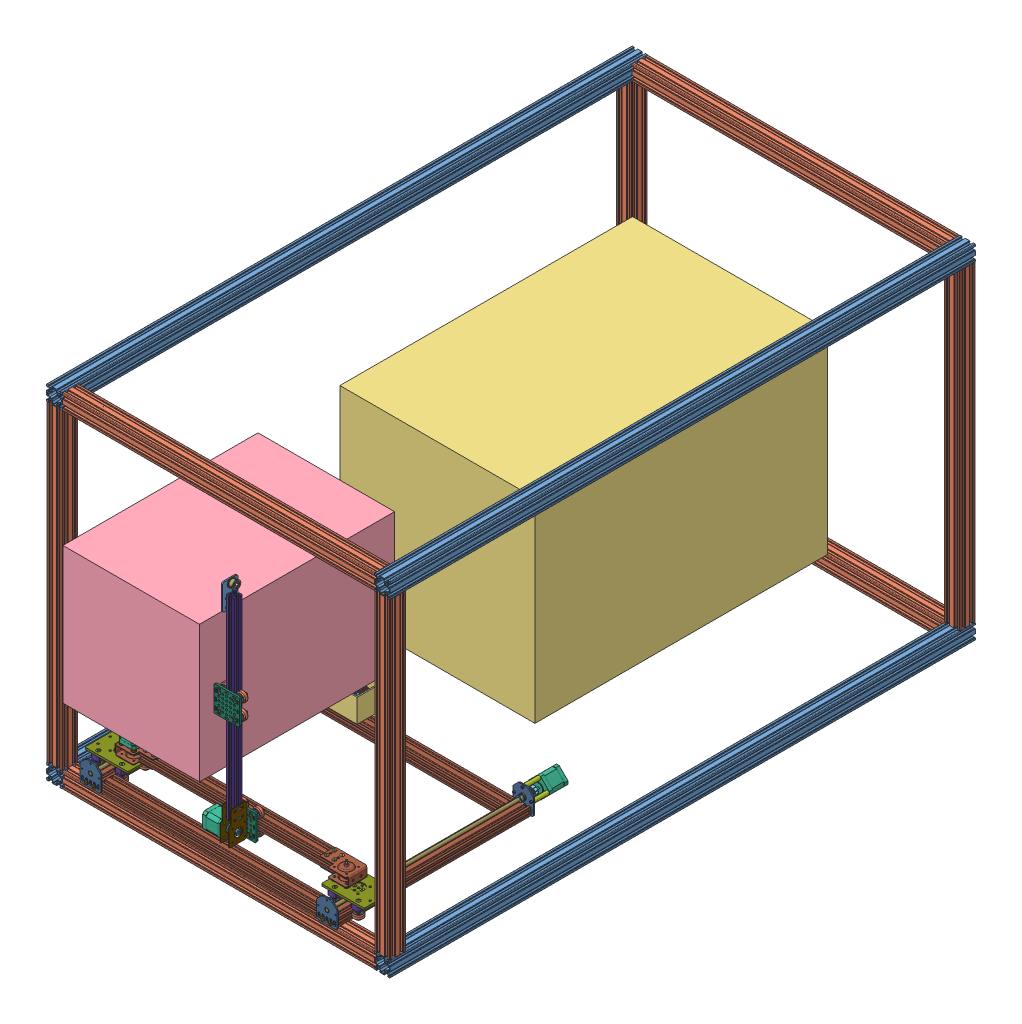
SolidWorks assembly box, configuration 預設. Lengths in mm.
Overall size (880 880 1515.78).
295 component instances, 42 part files, 42 mates.
Components (placement in the parent):
- V-Slot 40x40x1500 Linear Rail-1: V-Slot 40x40x1500 Linear Rail [Default] at (-19.0751 -0.7358 750) size (40 40 1500)
- V-Slot 40x40x1500 Linear Rail-2: V-Slot 40x40x1500 Linear Rail [Default] at (-19.0751 -840.7358 750) size (40 40 1500)
- V-Slot 40x40x1000 Linear Rail-1: V-Slot 40x40x1000 Linear Rail [40 x 40 x 800] at (-19.0751 -820.7358 2230) x (0 0 1) z (0 1 0) size (40 40 800)
- V-Slot 40x40x1000 Linear Rail-2: V-Slot 40x40x1000 Linear Rail [40 x 40 x 800] at (-19.0751 -820.7358 770) x (1 0 0) z (0 1 0) size (40 40 800)
- V-Slot 40x40x1000 Linear Rail-3: V-Slot 40x40x1000 Linear Rail [40 x 40 x 800] at (800.9249 -840.7358 2230) x (0 0 1) z (-1 0 0) size (40 40 800)
- V-Slot 40x40x1000 Linear Rail-4: V-Slot 40x40x1000 Linear Rail [40 x 40 x 800] at (800.9249 -0.7358 2230) x (0 0 1) z (-1 0 0) size (40 40 800)
- V-Slot 40x40x1000 Linear Rail-7: V-Slot 40x40x1000 Linear Rail [40 x 40 x 800] at (820.9249 -20.7358 2230) x (1 0 0) z (0 -1 0) size (40 40 800)
- V-Slot 40x40x1000 Linear Rail-8: V-Slot 40x40x1000 Linear Rail [40 x 40 x 800] at (800.9249 -840.7358 770) x (0 0 1) z (-1 0 0) size (40 40 800)
- V-Slot 40x40x1000 Linear Rail-9: V-Slot 40x40x1000 Linear Rail [40 x 40 x 800] at (820.9249 -820.7358 770) x (1 0 0) z (0 1 0) size (40 40 800)
- V-Slot 40x40x1000 Linear Rail-10: V-Slot 40x40x1000 Linear Rail [40 x 40 x 800] at (800.9249 -0.7358 770) x (0 0 1) z (-1 0 0) size (40 40 800)
- V-Slot 40x40x1500 Linear Rail-5: V-Slot 40x40x1500 Linear Rail [Default] at (820.9249 -840.7358 750) size (40 40 1500)
- V-Slot 40x40x1500 Linear Rail-6: V-Slot 40x40x1500 Linear Rail [Default] at (820.9249 -0.7358 750) size (40 40 1500)
- frige-2: frige [RS-5075G] at (307.8977 -579.3938 788.5) size (500 500 750)
- oven-1: oven [預設] at (0.9249 -15184.575 11029.75) x (0 -1 0) z (1 0 0) size (350 500 350)
- keg-1: keg [12L] at (296.649 -568.3878 823.5037) size (226.6 226.6 413)
- manipulator2-1: manipulator2 [預設] at (654.9752 -796.101 2551.2052) x (-0.998451 -0.052967 0.017023) z (-0.017075 0.000534 -0.999854) size (716.52 632.64 604.45) (flexible)
  - Button Head Socket Cap Screw M3-1: Button Head Socket Cap Screw M3 [M3 x 17] at (-17.8347 8.2677 364.2512) x (0.052967 -0.998596 -0.000534) z (0.000534 -0.000506 1) size (18.72 5.7 5.7)
  - Button Head Socket Cap Screw M3-2: Button Head Socket Cap Screw M3 [M3 x 17] at (13.1173 9.9092 364.7806) x (0.052967 -0.998596 -0.000534) z (0.000534 -0.000506 1) size (18.72 5.7 5.7)
  - Button Head Socket Cap Screw M3-3: Button Head Socket Cap Screw M3 [M3 x 17] at (-18.3624 8.2232 395.2467) x (0.052967 -0.998596 -0.000534) z (0.000534 -0.000506 1) size (18.72 5.7 5.7)
  - Button Head Socket Cap Screw M3-4: Button Head Socket Cap Screw M3 [M3 x 17] at (12.5896 9.8646 395.776) x (0.052967 -0.998596 -0.000534) z (0.000534 -0.000506 1) size (18.72 5.7 5.7)
  - Nylon Insert Lock Nut M3-3: Nylon Insert Lock Nut M3 [Default] at (12.8843 14.303 364.7829) x (-0.998393 -0.052967 0.02015) z (0.02015 0.000534 0.999797) size (5.5 4 6.35)
  - Nylon Insert Lock Nut M3-4: Nylon Insert Lock Nut M3 [Default] at (12.3566 14.2584 395.7784) x (-0.998393 -0.052967 0.02015) z (0.02015 0.000534 0.999797) size (5.5 4 6.35)
  - Nylon Insert Lock Nut M3-5: Nylon Insert Lock Nut M3 [Default] at (-18.5954 12.617 395.2491) x (-0.998393 -0.052967 0.02015) z (0.02015 0.000534 0.999797) size (5.5 4 6.35)
  - Nylon Insert Lock Nut M3-6: Nylon Insert Lock Nut M3 [Default] at (-18.0677 12.6615 364.2536) x (-0.998393 -0.052967 0.02015) z (0.02015 0.000534 0.999797) size (5.5 4 6.35)
  - Aluminum Spacer 3mm-1: Aluminum Spacer 3mm [6mm] at (12.3016 25.2875 364.7888) x (0.997193 0.05292 -0.052967) z (0.052967 -0.998596 -0.000534) size (10 10 6)
  - Aluminum Spacer 3mm-2: Aluminum Spacer 3mm [6mm] at (-18.6504 23.6461 364.2595) x (0.997193 0.05292 -0.052967) z (0.052967 -0.998596 -0.000534) size (10 10 6)
  - Aluminum Spacer 3mm-3: Aluminum Spacer 3mm [6mm] at (-19.1781 23.6015 395.2549) x (0.997193 0.05292 -0.052967) z (0.052967 -0.998596 -0.000534) size (10 10 6)
  - Aluminum Spacer 3mm-4: Aluminum Spacer 3mm [6mm] at (11.7739 25.243 395.7843) x (0.997193 0.05292 -0.052967) z (0.052967 -0.998596 -0.000534) size (10 10 6)
  - Z2-1: Z2 [Default] at (-565.1545 -15.5578 336.9084) size (111.46 63.72 594.1) (flexible)
    - Ball Bearing 8 x 16 x 5-4: Ball Bearing 8 x 16 x 5 [Default] at (533.6792 21.533 -34.6863) x (-0.017023 -0.001438 0.999854) z (-0.57924 -0.815083 -0.011034) size (5 16 16)
    - Threaded Rod Plate Nema 17-3: Threaded Rod Plate Nema 17 [Default] at (533.7388 21.538 -38.1858) x (0.998451 0.05295 0.017075) z (0.052967 -0.998596 -0.000534) size (53 3 59.29)
    - V-Slot 20x40x500 Linear Rail-1: V-Slot 20x40x500 Linear Rail [Default] at (534.8758 -0.8648 -35.1982) x (0.052967 -0.998596 -0.000534) z (-0.017023 -0.001438 0.999854) size (20 40 500)
    - Threaded Rod Plate Nema 17-6: Threaded Rod Plate Nema 17 [Default] at (525.1253 20.8106 467.7404) x (-0.998451 -0.05295 -0.017075) z (0.052967 -0.998596 -0.000534) size (53 3 59.29)
    - Ball Bearing 8 x 16 x 5-6: Ball Bearing 8 x 16 x 5 [Default] at (525.1849 20.8156 464.2409) x (0.017023 0.001438 -0.999854) z (0.999854 0.001413 0.017025) size (5 16 16)
    - 8mm leadscrew 540mm-1: 8mm leadscrew 540mm [520mm] at (533.7388 21.538 -38.1858) x (-0.290929 0.956738 -0.003577) z (-0.017023 -0.001438 0.999854) size (8 8 520)
    - Shim Washer 8mm-5: Shim Washer 8mm [Default] at (525.2274 20.8192 461.7412) x (0.999711 -0.017023 0.016996) z (0.016996 0.999854 0.001727) size (11.8 1.15 11.8)
    - Shim Washer 8mm-6: Shim Washer 8mm [Default] at (533.6367 21.5294 -32.1867) x (0.99971 0.017023 0.017045) z (0.017045 -0.999854 -0.001147) size (11.8 1.15 11.8)
    - Lock Collar 8mm-5: Lock Collar 8mm [Default] at (525.3662 20.8309 453.5924) x (0.999855 -0.000012 0.017023) z (-0.017023 -0.001438 0.999854) size (14 14 7)
    - Lock Collar 8mm-6: Lock Collar 8mm [Default] at (533.6171 21.5277 -31.0369) x (0.999855 -0.000012 0.017023) z (-0.017023 -0.001438 0.999854) size (14 14 7)
    - 8mm Acme Nut Block-3: 8mm Acme Nut Block [Default] at (532.5339 21.4362 32.5885) x (-0.998451 -0.05295 -0.017075) z (-0.017023 -0.001438 0.999854) size (34 12 20)
    - mid plate-3: mid plate [預設] at (529.8068 31.4237 -84.4607) x (0.998451 0.05295 0.017075) z (-0.017023 -0.001438 0.999854) size (110 42 86.72)
      - V-Slot Gantry Plate 20-80mm 2-1: V-Slot Gantry Plate 20-80mm 2 [Default] at (4.1926 -4.0553 127) size (110 5 80)
      - Spacer Block 2-1: Spacer Block 2 [Default] at (-26.1074 -16.0553 127) x (0 0 -1) z (0 1 0) size (80 20 12)
      - Spacer Block 2-2: Spacer Block 2 [Default] at (34.4926 -16.0553 127) x (0 0 -1) z (0 1 0) size (80 20 12)
      - Aluminum Spacer 6mm-1: Aluminum Spacer 6mm [9mm] at (34.4926 -25.0553 97) x (1 0 0) z (0 1 0) size (10 10 9)
      - Aluminum Spacer 6mm-2: Aluminum Spacer 6mm [9mm] at (34.4926 -25.0553 157) x (1 0 0) z (0 1 0) size (10 10 9)
      - Aluminum Spacer 6mm-3: Aluminum Spacer 6mm [9mm] at (-26.1074 -25.0553 97) x (1 0 0) z (0 1 0) size (10 10 9)
      - Aluminum Spacer 6mm-4: Aluminum Spacer 6mm [9mm] at (-26.1074 -25.0553 157) x (1 0 0) z (0 1 0) size (10 10 9)
      - small wheel-9: small wheel [預設] at (-14.754 -38.612 99.7479) x (0 -1 0) z (0 0 1) size (11 23.9 23.9)
        - Ball Bearing 5 x 16 x 5-2: Ball Bearing 5 x 16 x 5 [Default] at (-5.0567 -11.3534 -2.7479) size (5 16 16)
        - Solid V Wheel-2: Solid V Wheel [Default] at (-8.0567 -11.3534 -2.7479) size (10.2 23.9 23.9)
        - Ball Bearing 5 x 16 x 5-3: Ball Bearing 5 x 16 x 5 [Default] at (-11.0567 -11.3534 -2.7479) size (5 16 16)
      - small wheel-10: small wheel [預設] at (-14.4269 -38.612 156.8676) x (0 -1 0) z (0.246245 0 0.969207) size (11 23.9 23.9)
        - Ball Bearing 5 x 16 x 5-2: Ball Bearing 5 x 16 x 5 [Default] at (-5.0567 -11.3534 -2.7479) size (5 16 16)
        - Solid V Wheel-2: Solid V Wheel [Default] at (-8.0567 -11.3534 -2.7479) size (10.2 23.9 23.9)
        - Ball Bearing 5 x 16 x 5-3: Ball Bearing 5 x 16 x 5 [Default] at (-11.0567 -11.3534 -2.7479) size (5 16 16)
      - small wheel-11: small wheel [預設] at (46.169 -38.612 156.6628) x (0 -1 0) z (0.263197 0 0.964742) size (11 23.9 23.9)
        - Ball Bearing 5 x 16 x 5-2: Ball Bearing 5 x 16 x 5 [Default] at (-5.0567 -11.3534 -2.7479) size (5 16 16)
        - Solid V Wheel-2: Solid V Wheel [Default] at (-8.0567 -11.3534 -2.7479) size (10.2 23.9 23.9)
        - Ball Bearing 5 x 16 x 5-3: Ball Bearing 5 x 16 x 5 [Default] at (-11.0567 -11.3534 -2.7479) size (5 16 16)
      - small wheel-12: small wheel [預設] at (45.8243 -38.612 99.8362) x (0 -1 0) z (-0.007785 0 0.99997) size (11 23.9 23.9)
        - Ball Bearing 5 x 16 x 5-2: Ball Bearing 5 x 16 x 5 [Default] at (-5.0567 -11.3534 -2.7479) size (5 16 16)
        - Solid V Wheel-2: Solid V Wheel [Default] at (-8.0567 -11.3534 -2.7479) size (10.2 23.9 23.9)
        - Ball Bearing 5 x 16 x 5-3: Ball Bearing 5 x 16 x 5 [Default] at (-11.0567 -11.3534 -2.7479) size (5 16 16)
      - Low Profile Screw M5-6: Low Profile Screw M5 [M5 x 40] at (-26.1074 -41.0553 157) x (0 -1 0) z (0 0 1) size (41.62 9 9)
      - Low Profile Screw M5-7: Low Profile Screw M5 [M5 x 40] at (-26.1074 -41.0553 97) x (0 -1 0) z (0 0 1) size (41.62 9 9)
      - Low Profile Screw M5-8: Low Profile Screw M5 [M5 x 40] at (34.4926 -41.0553 97) x (0 -1 0) z (0 0 1) size (41.62 9 9)
      - Low Profile Screw M5-10: Low Profile Screw M5 [M5 x 40] at (34.4926 -41.0553 157) x (0 -1 0) z (0 0 1) size (41.62 9 9)
      - Nylon Insert Lock Nut M5-5: Nylon Insert Lock Nut M5 [Default] at (-26.1074 -36.0553 157) x (0.837169 0 0.546944) z (0.546944 0 -0.837169) size (8 5 9.24)
      - Nylon Insert Lock Nut M5-6: Nylon Insert Lock Nut M5 [Default] at (-26.1074 -36.0553 97) x (0.837169 0 0.546944) z (0.546944 0 -0.837169) size (8 5 9.24)
      - Nylon Insert Lock Nut M5-7: Nylon Insert Lock Nut M5 [Default] at (34.4926 -36.0553 157) x (0.837169 0 0.546944) z (0.546944 0 -0.837169) size (8 5 9.24)
      - Nylon Insert Lock Nut M5-8: Nylon Insert Lock Nut M5 [Default] at (34.4926 -36.0553 97) x (0.837169 0 0.546944) z (0.546944 0 -0.837169) size (8 5 9.24)
    - Flexible Coupling 5mm x 8mm-4: Flexible Coupling 5mm x 8mm [Default] at (524.6742 20.7725 494.2365) x (-0.433195 0.90128 -0.006079) z (-0.017023 -0.001438 0.999854) size (21.03 20 25)
    - Nema 17 Stepper Motor-3: Nema 17 Stepper Motor [Default] at (524.4784 20.7559 505.7348) x (-0.743465 0.668673 -0.011696) z (0.017023 0.001438 -0.999854) size (42.42 42.42 72)
    - Aluminum Spacer 40mm-5: Aluminum Spacer 40mm [38] at (546.3648 21.9166 506.1091) x (-0.985691 -0.1677 -0.017023) z (0.017023 0.001438 -0.999854) size (10 10 38)
    - Aluminum Spacer 40mm-6: Aluminum Spacer 40mm [38] at (523.3174 42.6455 505.7465) x (-0.985691 -0.1677 -0.017023) z (0.017023 0.001438 -0.999854) size (10 10 38)
    - Aluminum Spacer 40mm-7: Aluminum Spacer 40mm [38] at (502.5921 19.5953 505.3605) x (-0.985691 -0.1677 -0.017023) z (0.017023 0.001438 -0.999854) size (10 10 38)
    - Socket Head Cap Screw M3-8: Socket Head Cap Screw M3 [M3 x 45] at (523.2493 42.6397 509.7459) x (-0.017023 -0.001438 0.999854) z (-0.999854 0.001462 -0.017021) size (48.09 5.5 5.5)
    - Socket Head Cap Screw M3-9: Socket Head Cap Screw M3 [M3 x 45] at (502.524 19.5895 509.3599) x (-0.017023 -0.001438 0.999854) z (-0.999854 0.001462 -0.017021) size (48.09 5.5 5.5)
    - Socket Head Cap Screw M3-10: Socket Head Cap Screw M3 [M3 x 45] at (546.2967 21.9109 510.1085) x (-0.017023 -0.001438 0.999854) z (-0.999854 0.001462 -0.017021) size (48.09 5.5 5.5)
    - Self Tapping Screw-1: Self Tapping Screw [Default] at (536.371 -2.4365 467.8984) x (0.99971 0.017023 0.017045) z (0.017045 -0.999854 -0.001147) size (9.6 20.4 9.6)
    - Self Tapping Screw-2: Self Tapping Screw [Default] at (516.4019 -3.4955 467.5569) x (0.99971 0.017023 0.017045) z (0.017045 -0.999854 -0.001147) size (9.6 20.4 9.6)
    - Self Tapping Screw-3: Self Tapping Screw [Default] at (544.9844 -1.7091 -38.0278) x (0.999711 -0.017023 0.016996) z (0.016996 0.999854 0.001727) size (9.6 20.4 9.6)
    - Self Tapping Screw-4: Self Tapping Screw [Default] at (525.0154 -2.7681 -38.3693) x (0.999711 -0.017023 0.016996) z (0.016996 0.999854 0.001727) size (9.6 20.4 9.6)
    - Nylon Insert Lock Nut M5-1: Nylon Insert Lock Nut M5 [Default] at (542.4011 20.9528 42.7572) x (-0.998393 -0.052967 0.02015) z (0.02015 0.000534 0.999797) size (8 5 9.24)
    - Nylon Insert Lock Nut M5-2: Nylon Insert Lock Nut M5 [Default] at (522.4321 19.8938 42.4157) x (-0.998393 -0.052967 0.02015) z (0.02015 0.000534 0.999797) size (8 5 9.24)
    - Low Profile Screw M5-1: Low Profile Screw M5 [M5 x 15] at (542.6659 15.9598 42.7546) x (0.052967 -0.998596 -0.000534) z (0.000534 -0.000506 1) size (16.62 9 9)
    - Low Profile Screw M5-2: Low Profile Screw M5 [M5 x 15] at (522.6969 14.9008 42.4131) x (0.052967 -0.998596 -0.000534) z (0.000534 -0.000506 1) size (16.62 9 9)
  - V-Slot 20x40x500 Linear Rail-1: V-Slot 20x40x500 Linear Rail [20 x 40 x 566] at (554.3834 14.5723 331.7116) x (-0.052967 0.998596 0.000534) z (-0.998451 -0.05295 -0.017075) size (20 40 565.91)
  - V-Slot 20x40x500 Linear Rail-2: V-Slot 20x40x500 Linear Rail [20 x 40 x 566] at (546.5529 13.911 791.6445) x (-0.052967 0.998596 0.000534) z (-0.998451 -0.05295 -0.017075) size (20 40 565.91)
  - Z2-4: Z2 [Default] at (39.9069 16.5297 347.2558) size (111.46 63.72 594.1) (flexible)
    - Ball Bearing 8 x 16 x 5-4: Ball Bearing 8 x 16 x 5 [Default] at (533.6792 21.533 -34.6863) x (-0.017023 -0.001438 0.999854) z (-0.57924 -0.815083 -0.011034) size (5 16 16)
    - Threaded Rod Plate Nema 17-3: Threaded Rod Plate Nema 17 [Default] at (533.7388 21.538 -38.1858) x (0.998451 0.05295 0.017075) z (0.052967 -0.998596 -0.000534) size (53 3 59.29)
    - V-Slot 20x40x500 Linear Rail-1: V-Slot 20x40x500 Linear Rail [Default] at (534.8758 -0.8648 -35.1982) x (0.052967 -0.998596 -0.000534) z (-0.017023 -0.001438 0.999854) size (20 40 500)
    - Threaded Rod Plate Nema 17-6: Threaded Rod Plate Nema 17 [Default] at (525.1253 20.8106 467.7404) x (-0.998451 -0.05295 -0.017075) z (0.052967 -0.998596 -0.000534) size (53 3 59.29)
    - Ball Bearing 8 x 16 x 5-6: Ball Bearing 8 x 16 x 5 [Default] at (525.1849 20.8156 464.2409) x (0.017023 0.001438 -0.999854) z (0.999854 0.001413 0.017025) size (5 16 16)
    - 8mm leadscrew 540mm-1: 8mm leadscrew 540mm [520mm] at (533.7388 21.538 -38.1858) x (-0.290929 0.956738 -0.003577) z (-0.017023 -0.001438 0.999854) size (8 8 520)
    - Shim Washer 8mm-5: Shim Washer 8mm [Default] at (525.2274 20.8192 461.7412) x (0.999711 -0.017023 0.016996) z (0.016996 0.999854 0.001727) size (11.8 1.15 11.8)
    - Shim Washer 8mm-6: Shim Washer 8mm [Default] at (533.6367 21.5294 -32.1867) x (0.99971 0.017023 0.017045) z (0.017045 -0.999854 -0.001147) size (11.8 1.15 11.8)
    - Lock Collar 8mm-5: Lock Collar 8mm [Default] at (525.3662 20.8309 453.5924) x (0.999855 -0.000012 0.017023) z (-0.017023 -0.001438 0.999854) size (14 14 7)
    - Lock Collar 8mm-6: Lock Collar 8mm [Default] at (533.6171 21.5277 -31.0369) x (0.999855 -0.000012 0.017023) z (-0.017023 -0.001438 0.999854) size (14 14 7)
    - 8mm Acme Nut Block-3: 8mm Acme Nut Block [Default] at (532.5339 21.4362 32.5885) x (-0.998451 -0.05295 -0.017075) z (-0.017023 -0.001438 0.999854) size (34 12 20)
    - mid plate-3: mid plate [預設] at (529.8068 31.4237 -84.4607) x (0.998451 0.05295 0.017075) z (-0.017023 -0.001438 0.999854) size (110 42 86.72)
      - V-Slot Gantry Plate 20-80mm 2-1: V-Slot Gantry Plate 20-80mm 2 [Default] at (4.1926 -4.0553 127) size (110 5 80)
      - Spacer Block 2-1: Spacer Block 2 [Default] at (-26.1074 -16.0553 127) x (0 0 -1) z (0 1 0) size (80 20 12)
      - Spacer Block 2-2: Spacer Block 2 [Default] at (34.4926 -16.0553 127) x (0 0 -1) z (0 1 0) size (80 20 12)
      - Aluminum Spacer 6mm-1: Aluminum Spacer 6mm [9mm] at (34.4926 -25.0553 97) x (1 0 0) z (0 1 0) size (10 10 9)
      - Aluminum Spacer 6mm-2: Aluminum Spacer 6mm [9mm] at (34.4926 -25.0553 157) x (1 0 0) z (0 1 0) size (10 10 9)
      - Aluminum Spacer 6mm-3: Aluminum Spacer 6mm [9mm] at (-26.1074 -25.0553 97) x (1 0 0) z (0 1 0) size (10 10 9)
      - Aluminum Spacer 6mm-4: Aluminum Spacer 6mm [9mm] at (-26.1074 -25.0553 157) x (1 0 0) z (0 1 0) size (10 10 9)
      - small wheel-9: small wheel [預設] at (-14.754 -38.612 99.7479) x (0 -1 0) z (0 0 1) size (11 23.9 23.9)
        - Ball Bearing 5 x 16 x 5-2: Ball Bearing 5 x 16 x 5 [Default] at (-5.0567 -11.3534 -2.7479) size (5 16 16)
        - Solid V Wheel-2: Solid V Wheel [Default] at (-8.0567 -11.3534 -2.7479) size (10.2 23.9 23.9)
        - Ball Bearing 5 x 16 x 5-3: Ball Bearing 5 x 16 x 5 [Default] at (-11.0567 -11.3534 -2.7479) size (5 16 16)
      - small wheel-10: small wheel [預設] at (-14.4269 -38.612 156.8676) x (0 -1 0) z (0.246245 0 0.969207) size (11 23.9 23.9)
        - Ball Bearing 5 x 16 x 5-2: Ball Bearing 5 x 16 x 5 [Default] at (-5.0567 -11.3534 -2.7479) size (5 16 16)
        - Solid V Wheel-2: Solid V Wheel [Default] at (-8.0567 -11.3534 -2.7479) size (10.2 23.9 23.9)
        - Ball Bearing 5 x 16 x 5-3: Ball Bearing 5 x 16 x 5 [Default] at (-11.0567 -11.3534 -2.7479) size (5 16 16)
      - small wheel-11: small wheel [預設] at (46.169 -38.612 156.6628) x (0 -1 0) z (0.263197 0 0.964742) size (11 23.9 23.9)
        - Ball Bearing 5 x 16 x 5-2: Ball Bearing 5 x 16 x 5 [Default] at (-5.0567 -11.3534 -2.7479) size (5 16 16)
        - Solid V Wheel-2: Solid V Wheel [Default] at (-8.0567 -11.3534 -2.7479) size (10.2 23.9 23.9)
        - Ball Bearing 5 x 16 x 5-3: Ball Bearing 5 x 16 x 5 [Default] at (-11.0567 -11.3534 -2.7479) size (5 16 16)
      - small wheel-12: small wheel [預設] at (45.8243 -38.612 99.8362) x (0 -1 0) z (-0.007785 0 0.99997) size (11 23.9 23.9)
        - Ball Bearing 5 x 16 x 5-2: Ball Bearing 5 x 16 x 5 [Default] at (-5.0567 -11.3534 -2.7479) size (5 16 16)
        - Solid V Wheel-2: Solid V Wheel [Default] at (-8.0567 -11.3534 -2.7479) size (10.2 23.9 23.9)
        - Ball Bearing 5 x 16 x 5-3: Ball Bearing 5 x 16 x 5 [Default] at (-11.0567 -11.3534 -2.7479) size (5 16 16)
      - Low Profile Screw M5-6: Low Profile Screw M5 [M5 x 40] at (-26.1074 -41.0553 157) x (0 -1 0) z (0 0 1) size (41.62 9 9)
      - Low Profile Screw M5-7: Low Profile Screw M5 [M5 x 40] at (-26.1074 -41.0553 97) x (0 -1 0) z (0 0 1) size (41.62 9 9)
      - Low Profile Screw M5-8: Low Profile Screw M5 [M5 x 40] at (34.4926 -41.0553 97) x (0 -1 0) z (0 0 1) size (41.62 9 9)
      - Low Profile Screw M5-10: Low Profile Screw M5 [M5 x 40] at (34.4926 -41.0553 157) x (0 -1 0) z (0 0 1) size (41.62 9 9)
      - Nylon Insert Lock Nut M5-5: Nylon Insert Lock Nut M5 [Default] at (-26.1074 -36.0553 157) x (0.837169 0 0.546944) z (0.546944 0 -0.837169) size (8 5 9.24)
      - Nylon Insert Lock Nut M5-6: Nylon Insert Lock Nut M5 [Default] at (-26.1074 -36.0553 97) x (0.837169 0 0.546944) z (0.546944 0 -0.837169) size (8 5 9.24)
      - Nylon Insert Lock Nut M5-7: Nylon Insert Lock Nut M5 [Default] at (34.4926 -36.0553 157) x (0.837169 0 0.546944) z (0.546944 0 -0.837169) size (8 5 9.24)
      - Nylon Insert Lock Nut M5-8: Nylon Insert Lock Nut M5 [Default] at (34.4926 -36.0553 97) x (0.837169 0 0.546944) z (0.546944 0 -0.837169) size (8 5 9.24)
    - Flexible Coupling 5mm x 8mm-4: Flexible Coupling 5mm x 8mm [Default] at (524.6742 20.7725 494.2365) x (-0.433195 0.90128 -0.006079) z (-0.017023 -0.001438 0.999854) size (21.03 20 25)
    - Nema 17 Stepper Motor-3: Nema 17 Stepper Motor [Default] at (524.4784 20.7559 505.7348) x (-0.743465 0.668673 -0.011696) z (0.017023 0.001438 -0.999854) size (42.42 42.42 72)
    - Aluminum Spacer 40mm-5: Aluminum Spacer 40mm [38] at (546.3648 21.9166 506.1091) x (-0.985691 -0.1677 -0.017023) z (0.017023 0.001438 -0.999854) size (10 10 38)
    - Aluminum Spacer 40mm-6: Aluminum Spacer 40mm [38] at (523.3174 42.6455 505.7465) x (-0.985691 -0.1677 -0.017023) z (0.017023 0.001438 -0.999854) size (10 10 38)
    - Aluminum Spacer 40mm-7: Aluminum Spacer 40mm [38] at (502.5921 19.5953 505.3605) x (-0.985691 -0.1677 -0.017023) z (0.017023 0.001438 -0.999854) size (10 10 38)
    - Socket Head Cap Screw M3-8: Socket Head Cap Screw M3 [M3 x 45] at (523.2493 42.6397 509.7459) x (-0.017023 -0.001438 0.999854) z (-0.999854 0.001462 -0.017021) size (48.09 5.5 5.5)
    - Socket Head Cap Screw M3-9: Socket Head Cap Screw M3 [M3 x 45] at (502.524 19.5895 509.3599) x (-0.017023 -0.001438 0.999854) z (-0.999854 0.001462 -0.017021) size (48.09 5.5 5.5)
    - Socket Head Cap Screw M3-10: Socket Head Cap Screw M3 [M3 x 45] at (546.2967 21.9109 510.1085) x (-0.017023 -0.001438 0.999854) z (-0.999854 0.001462 -0.017021) size (48.09 5.5 5.5)
    - Self Tapping Screw-1: Self Tapping Screw [Default] at (536.371 -2.4365 467.8984) x (0.99971 0.017023 0.017045) z (0.017045 -0.999854 -0.001147) size (9.6 20.4 9.6)
    - Self Tapping Screw-2: Self Tapping Screw [Default] at (516.4019 -3.4955 467.5569) x (0.99971 0.017023 0.017045) z (0.017045 -0.999854 -0.001147) size (9.6 20.4 9.6)
    - Self Tapping Screw-3: Self Tapping Screw [Default] at (544.9844 -1.7091 -38.0278) x (0.999711 -0.017023 0.016996) z (0.016996 0.999854 0.001727) size (9.6 20.4 9.6)
    - Self Tapping Screw-4: Self Tapping Screw [Default] at (525.0154 -2.7681 -38.3693) x (0.999711 -0.017023 0.016996) z (0.016996 0.999854 0.001727) size (9.6 20.4 9.6)
    - Nylon Insert Lock Nut M5-1: Nylon Insert Lock Nut M5 [Default] at (542.4011 20.9528 42.7572) x (-0.998393 -0.052967 0.02015) z (0.02015 0.000534 0.999797) size (8 5 9.24)
    - Nylon Insert Lock Nut M5-2: Nylon Insert Lock Nut M5 [Default] at (522.4321 19.8938 42.4157) x (-0.998393 -0.052967 0.02015) z (0.02015 0.000534 0.999797) size (8 5 9.24)
    - Low Profile Screw M5-1: Low Profile Screw M5 [M5 x 15] at (542.6659 15.9598 42.7546) x (0.052967 -0.998596 -0.000534) z (0.000534 -0.000506 1) size (16.62 9 9)
    - Low Profile Screw M5-2: Low Profile Screw M5 [M5 x 15] at (522.6969 14.9008 42.4131) x (0.052967 -0.998596 -0.000534) z (0.000534 -0.000506 1) size (16.62 9 9)
  - Y-1: Y [Default] at (-53.9338 467.0765 1482.6584) x (0.061515 -0.998106 -0.000537) z (0.998106 0.061515 -0.00018) size (96.37 65.23 599.86) (flexible)
    - Aluminum Spacer 6mm-1: Aluminum Spacer 6mm [Default] at (421.0945 1108.215 584.4034) x (0.00697 0.580866 0.813969) z (0.999963 -0.000001 -0.008562) size (10 10 6)
    - Aluminum Spacer 6mm-2: Aluminum Spacer 6mm [Default] at (427.0897 1077.2197 583.817) x (-0.008174 0.297659 -0.954637) z (-0.999963 0.000001 0.008562) size (10 10 6)
    - Aluminum Spacer 6mm-3: Aluminum Spacer 6mm [Default] at (426.8289 1108.7501 553.3578) x (-0.008322 0.234979 -0.971965) z (-0.999963 0.000001 0.008562) size (10 10 6)
    - Aluminum Spacer 6mm-4: Aluminum Spacer 6mm [Default] at (420.8245 1077.7547 552.8741) x (0.003973 0.88592 0.463821) z (0.999963 -0.000001 -0.008562) size (10 10 6)
    - Aluminum Spacer 6mm-7: Aluminum Spacer 6mm [Default] at (446.3917 1102.3933 23.3622) x (0.008562 0.000001 0.999963) z (-0.999963 0.000001 0.008562) size (10 10 6)
    - Aluminum Spacer 6mm-8: Aluminum Spacer 6mm [Default] at (427.2924 1102.3934 23.5258) x (0.00638 -0.666766 0.74524) z (-0.999963 0.000001 0.008562) size (10 10 6)
    - Button Head Socket Cap Screw M3-2: Button Head Socket Cap Screw M3 [M3 x 12] at (416.6947 1108.2151 584.4411) x (-0.999963 0.000001 0.008562) z (0.003271 0.924225 0.381835) size (13.72 5.7 5.7)
    - Button Head Socket Cap Screw M3-4: Button Head Socket Cap Screw M3 [M3 x 12] at (416.4247 1077.7547 552.9118) x (-0.999963 0.000001 0.008562) z (0.003271 0.924225 0.381835) size (13.72 5.7 5.7)
    - Button Head Socket Cap Screw M3-5: Button Head Socket Cap Screw M3 [M3 x 12] at (416.6901 1077.2197 583.906) x (-0.999963 0.000001 0.008562) z (0.003271 0.924225 0.381835) size (13.72 5.7 5.7)
    - Double Tee Nut-9: Double Tee Nut [Default] at (446.246 1069.0645 508.5583) x (0.008561 -0.01726 0.999814) z (-0.999963 0.000001 0.008562) size (36.88 10 3)
    - Double Tee Nut-14: Double Tee Nut [Default] at (446.249 1089.0615 508.9035) x (0.008561 -0.01726 0.999814) z (-0.999963 0.000001 0.008562) size (36.88 10 3)
    - Double Tee Nut-15: Double Tee Nut [Default] at (430.1623 1068.428 545.5719) x (-0.008561 0.01726 -0.999814) z (0.999963 -0.000001 -0.008562) size (36.88 10 3)
    - Double Tee Nut-16: Double Tee Nut [Default] at (430.1653 1088.425 545.917) x (-0.008561 0.01726 -0.999814) z (0.999963 -0.000001 -0.008562) size (36.88 10 3)
    - Double Tee Nut-20: Double Tee Nut [Default] at (426.2006 1096.4182 82.883) x (-0.008561 0.01726 -0.999814) z (0.999963 -0.000001 -0.008562) size (36.88 10 3)
    - Double Tee Nut-19: Double Tee Nut [Default] at (426.1976 1076.4212 82.5378) x (-0.008561 0.01726 -0.999814) z (0.999963 -0.000001 -0.008562) size (36.88 10 3)
    - Double Tee Nut-21: Double Tee Nut [Default] at (442.2842 1097.0547 45.8694) x (0.008561 -0.01726 0.999814) z (-0.999963 0.000001 0.008562) size (36.88 10 3)
    - Double Tee Nut-22: Double Tee Nut [Default] at (442.2813 1077.0577 45.5242) x (0.008561 -0.01726 0.999814) z (-0.999963 0.000001 0.008562) size (36.88 10 3)
    - Low Profile Screw M5-18: Low Profile Screw M5 [M5 x 6] at (428.729 1101.5631 74.5086) x (0.999963 -0.000001 -0.008562) z (0.003416 0.917023 0.398819) size (7.62 9 9)
    - Low Profile Screw M5-19: Low Profile Screw M5 [M5 x 6] at (428.726 1081.5661 74.1634) x (0.999963 -0.000001 -0.008562) z (0.006235 -0.685246 0.728285) size (7.62 9 9)
    - Low Profile Screw M5-20: Low Profile Screw M5 [M5 x 6] at (428.5548 1081.9113 54.1671) x (0.999963 -0.000001 -0.008562) z (-0.004605 -0.843137 -0.537678) size (7.62 9 9)
    - Low Profile Screw M5-21: Low Profile Screw M5 [M5 x 6] at (428.5577 1101.9083 54.5123) x (0.999963 -0.000001 -0.008562) z (-0.001108 -0.991612 -0.129244) size (7.62 9 9)
    - Low Profile Screw M5-22: Low Profile Screw M5 [M5 x 6] at (439.9285 1101.5631 74.4127) x (-0.999963 0.000001 0.008562) z (-0.008562 -0.000275 -0.999963) size (7.62 9 9)
    - Low Profile Screw M5-23: Low Profile Screw M5 [M5 x 6] at (439.7573 1101.9083 54.4164) x (-0.999963 0.000001 0.008562) z (-0.008562 -0.000275 -0.999963) size (7.62 9 9)
    - Low Profile Screw M5-24: Low Profile Screw M5 [M5 x 6] at (439.9256 1081.5661 74.0675) x (-0.999963 0.000001 0.008562) z (-0.008562 -0.000275 -0.999963) size (7.62 9 9)
    - Low Profile Screw M5-25: Low Profile Screw M5 [M5 x 6] at (439.7543 1081.9113 54.0712) x (-0.999963 0.000001 0.008562) z (-0.008562 -0.000275 -0.999963) size (7.62 9 9)
    - Low Profile Screw M5-26: Low Profile Screw M5 [M5 x 6] at (432.6937 1093.5699 537.5426) x (0.999963 -0.000001 -0.008562) z (0.008562 0 0.999963) size (7.62 9 9)
    - Low Profile Screw M5-28: Low Profile Screw M5 [M5 x 6] at (432.5195 1073.9181 517.2012) x (0.999963 -0.000001 -0.008562) z (0.008562 0 0.999963) size (7.62 9 9)
    - Low Profile Screw M5-29: Low Profile Screw M5 [M5 x 6] at (432.6907 1073.5729 537.1975) x (0.999963 -0.000001 -0.008562) z (0.008562 0 0.999963) size (7.62 9 9)
    - Low Profile Screw M5-30: Low Profile Screw M5 [M5 x 6] at (443.8933 1093.5699 537.4467) x (-0.999963 0.000001 0.008562) z (-0.006172 0.693056 -0.720857) size (7.62 9 9)
    - Low Profile Screw M5-31: Low Profile Screw M5 [M5 x 6] at (443.7221 1093.9151 517.4504) x (-0.999963 0.000001 0.008562) z (-0.007544 -0.473064 -0.880996) size (7.62 9 9)
    - Low Profile Screw M5-32: Low Profile Screw M5 [M5 x 6] at (443.8903 1073.5729 537.1016) x (-0.999963 0.000001 0.008562) z (-0.008393 -0.198144 -0.980137) size (7.62 9 9)
    - Low Profile Screw M5-33: Low Profile Screw M5 [M5 x 6] at (443.7191 1073.9181 517.1053) x (-0.999963 0.000001 0.008562) z (-0.005369 0.778884 -0.627145) size (7.62 9 9)
    - Low Profile Screw M5-34: Low Profile Screw M5 [M5 x 35] at (413.0929 1102.3934 23.6473) x (-0.999963 0.000001 0.008562) z (-0.007276 0.527011 -0.849827) size (36.62 9 9)
    - Nylon Insert Lock Nut M5-2: Nylon Insert Lock Nut M5 [Default] at (419.6927 1102.3934 23.5908) x (0.004535 0.848273 0.529539) z (0.007263 -0.529559 0.848242) size (8 5 9.24)
    - Low Profile Screw M5-35: Low Profile Screw M5 [M5 x 6] at (432.5225 1093.9151 517.5463) x (0.999963 -0.000001 -0.008562) z (0.008562 0 0.999963) size (7.62 9 9)
    - Button Head Socket Cap Screw M3-25: Button Head Socket Cap Screw M3 [M3 x 12] at (416.4293 1108.7501 553.4468) x (-0.999963 0.000001 0.008562) z (-0.008562 -0.000275 -0.999963) size (13.72 5.7 5.7)
    - Linear Actuator End Mount-1: Linear Actuator End Mount [Default] at (438.7777 1019.7292 594.0567) x (-0.999963 0.000001 0.008562) z (-0.008561 0.01726 -0.999814) size (28.4 54.9 86.33)
    - Linear Actuator End Mount-2: Linear Actuator End Mount [Default] at (433.6516 1030.0638 -4.6124) x (0.999963 -0.000001 -0.008562) z (0.008561 -0.01726 0.999814) size (28.4 54.9 86.33)
    - Nema 17 Stepper Motor-1: Nema 17 Stepper Motor [Default] at (420.9595 1092.9849 568.6388) x (-0.008561 0.01726 -0.999814) z (0.999963 -0.000001 -0.008562) size (42.42 42.42 72)
    - Smooth Idler-1: Smooth Idler [Default] at (433.8421 1102.3934 23.4697) x (0.999963 -0.000001 -0.008562) z (0.005218 -0.7928 0.609459) size (13.1 22 22)
      - Smooth Idler Pulley Wheel-1: Smooth Idler Pulley Wheel [Default] at origin size (12.7 22 22)
      - Ball Bearing 5 x 16 x 5-1: Ball Bearing 5 x 16 x 5 [Default] at (4.05 0 0) x (1 0 0) z (0 0.954651 0.297727) size (5 16 16)
      - Ball Bearing 5 x 16 x 5-2: Ball Bearing 5 x 16 x 5 [Default] at (-4.05 0 0) x (1 0 0) z (0 0.976216 -0.216802) size (5 16 16)
      - Nylon Spacer 0.125in-1: Nylon Spacer 0.125in [Default] at (-1.625 0 0) x (0 -0.24187 -0.970309) z (0 -0.970309 0.24187) size (7.94 3.17 7.94)
    - GT2 Timing Pulley 30 Tooth-1: GT2 Timing Pulley 30 Tooth [Default] at (426.6593 1092.9849 568.59) x (0.999963 -0.000001 -0.008562) z (-0.007129 -0.55389 -0.832559) size (17.5 22 22)
    - V-Slot 20x40x500 Linear Rail-1: V-Slot 20x40x500 Linear Rail [Default] at (434.0838 1092.0555 45.8533) x (0.999963 -0.000001 -0.008562) z (0.008561 -0.01726 0.999814) size (20 40 500)
    - small plate-2: small plate [預設] at (444.4301 1082.4312 227.4209) x (0.999761 -0.019668 -0.009529) z (0.009662 0.00665 0.999931) size (65.63 34.48 65.67)
      - small wheel-3: small wheel [預設] at (-0.7158 22.993 64.759) x (-0.019681 0.99952 0.023908) z (0.000235 -0.023908 0.999714) size (11 23.9 23.9)
        - Ball Bearing 5 x 16 x 5-2: Ball Bearing 5 x 16 x 5 [Default] at (-5.0567 -11.3534 -2.7479) size (5 16 16)
        - Solid V Wheel-2: Solid V Wheel [Default] at (-8.0567 -11.3534 -2.7479) size (10.2 23.9 23.9)
        - Ball Bearing 5 x 16 x 5-3: Ball Bearing 5 x 16 x 5 [Default] at (-11.0567 -11.3534 -2.7479) size (5 16 16)
      - small wheel-4: small wheel [預設] at (-40.708 22.2066 64.715) x (-0.019681 0.99952 0.023908) z (0.000235 -0.023908 0.999714) size (11 23.9 23.9)
        - Ball Bearing 5 x 16 x 5-2: Ball Bearing 5 x 16 x 5 [Default] at (-5.0567 -11.3534 -2.7479) size (5 16 16)
        - Solid V Wheel-2: Solid V Wheel [Default] at (-8.0567 -11.3534 -2.7479) size (10.2 23.9 23.9)
        - Ball Bearing 5 x 16 x 5-3: Ball Bearing 5 x 16 x 5 [Default] at (-11.0567 -11.3534 -2.7479) size (5 16 16)
      - V-Slot Gantry Plate 20mm 2-1: V-Slot Gantry Plate 20mm 2 [Default] at (-9.4756 29.8077 42.1523) x (0.999806 0.01966 0.0011) z (-0.000629 -0.023925 0.999714) size (65.5 5 65.5)
      - small wheel-5: small wheel [預設] at (-0.6906 23.95 24.7704) x (-0.019681 0.99952 0.023908) z (0.000235 -0.023908 0.999714) size (11 23.9 23.9)
        - Ball Bearing 5 x 16 x 5-2: Ball Bearing 5 x 16 x 5 [Default] at (-5.0567 -11.3534 -2.7479) size (5 16 16)
        - Solid V Wheel-2: Solid V Wheel [Default] at (-8.0567 -11.3534 -2.7479) size (10.2 23.9 23.9)
        - Ball Bearing 5 x 16 x 5-3: Ball Bearing 5 x 16 x 5 [Default] at (-11.0567 -11.3534 -2.7479) size (5 16 16)
      - small wheel-6: small wheel [預設] at (-40.6828 23.1636 24.7264) x (-0.019681 0.99952 0.023908) z (0.000235 -0.023908 0.999714) size (11 23.9 23.9)
        - Ball Bearing 5 x 16 x 5-2: Ball Bearing 5 x 16 x 5 [Default] at (-5.0567 -11.3534 -2.7479) size (5 16 16)
        - Solid V Wheel-2: Solid V Wheel [Default] at (-8.0567 -11.3534 -2.7479) size (10.2 23.9 23.9)
        - Ball Bearing 5 x 16 x 5-3: Ball Bearing 5 x 16 x 5 [Default] at (-11.0567 -11.3534 -2.7479) size (5 16 16)
      - Aluminum Spacer 9mm-1: Aluminum Spacer 9mm [Default] at (-29.3072 19.9403 61.9094) x (0.999806 0.019681 0.000235) z (-0.019681 0.99952 0.023908) size (10 10 9)
      - Aluminum Spacer 9mm-2: Aluminum Spacer 9mm [Default] at (10.6851 20.7267 61.9534) x (0.999806 0.019681 0.000235) z (-0.019681 0.99952 0.023908) size (10 10 9)
      - Aluminum Spacer 9mm-3: Aluminum Spacer 9mm [Default] at (-29.282 20.8973 21.9208) x (0.999806 0.019681 0.000235) z (-0.019681 0.99952 0.023908) size (10 10 9)
      - Aluminum Spacer 9mm-4: Aluminum Spacer 9mm [Default] at (10.7103 21.6837 21.9648) x (0.999806 0.019681 0.000235) z (-0.019681 0.99952 0.023908) size (10 10 9)
      - Low Profile Screw M5-7: Low Profile Screw M5 [M5 x 30] at (-28.9529 1.949 61.479) x (0.019681 -0.99952 -0.023908) z (0.000235 -0.023908 0.999714) size (31.62 9 9)
      - Low Profile Screw M5-8: Low Profile Screw M5 [M5 x 30] at (-28.9277 2.906 21.4905) x (0.019681 -0.99952 -0.023908) z (0.000235 -0.023908 0.999714) size (31.62 9 9)
      - Low Profile Screw M5-9: Low Profile Screw M5 [M5 x 30] at (11.0393 2.7354 61.523) x (0.019681 -0.99952 -0.023908) z (0.000235 -0.023908 0.999714) size (31.62 9 9)
      - Low Profile Screw M5-10: Low Profile Screw M5 [M5 x 30] at (11.0645 3.6924 21.5345) x (0.019681 -0.99952 -0.023908) z (0.000235 -0.023908 0.999714) size (31.62 9 9)
      - Nylon Insert Lock Nut M5-6: Nylon Insert Lock Nut M5 [Default] at (-29.0655 9.9026 21.6579) x (0.192329 -0.019681 0.981133) z (0.981133 0.023908 -0.191849) size (8 5 9.24)
      - Nylon Insert Lock Nut M5-7: Nylon Insert Lock Nut M5 [Default] at (-29.0907 8.9456 61.6464) x (0.192329 -0.019681 0.981133) z (0.981133 0.023908 -0.191849) size (8 5 9.24)
      - Nylon Insert Lock Nut M5-9: Nylon Insert Lock Nut M5 [Default] at (10.9016 9.732 61.6904) x (0.192329 -0.019681 0.981133) z (0.981133 0.023908 -0.191849) size (8 5 9.24)
      - Nylon Insert Lock Nut M5-10: Nylon Insert Lock Nut M5 [Default] at (10.9268 10.689 21.7018) x (0.192329 -0.019681 0.981133) z (0.981133 0.023908 -0.191849) size (8 5 9.24)
  - X-1: X [Default] at (379.6083 756.1782 632.5751) x (-0.998451 -0.05295 -0.017075) z (0.052967 -0.998596 -0.000534) size (92.45 47.68 584.07) (flexible)
    - Double Tee Nut-1: Double Tee Nut [Default] at (171.529 282.1788 684.0965) x (0 0 -1) z (1 0 0) size (36.88 10 3)
    - Double Tee Nut-2: Double Tee Nut [Default] at (171.529 282.1788 220.9765) x (0 0 -1) z (1 0 0) size (36.88 10 3)
    - Low Profile Screw M5-13: Low Profile Screw M5 [M5 x 25] at (190.729 287.1788 160.7465) size (26.62 9 9)
    - Nylon Insert Lock Nut M5-4: Nylon Insert Lock Nut M5 [Default] at (185.829 287.1788 160.7465) x (0 -1 0) z (0 0 1) size (8 5 9.24)
    - Low Profile Screw M5-14: Low Profile Screw M5 [M5 x 8] at (174.729 287.1788 192.5365) size (9.62 9 9)
    - Low Profile Screw M5-15: Low Profile Screw M5 [M5 x 8] at (174.729 287.1788 212.5365) size (9.62 9 9)
    - Button Head Socket Cap Screw M3-1: Button Head Socket Cap Screw M3 [M3 x 8] at (161.729 302.6788 691.1565) x (-1 0 0) z (0 0.924225 0.381849) size (9.72 5.7 5.7)
    - Button Head Socket Cap Screw M3-3: Button Head Socket Cap Screw M3 [M3 x 8] at (161.729 302.6788 722.1565) x (-1 0 0) z (0 0.924225 0.381849) size (9.72 5.7 5.7)
    - Button Head Socket Cap Screw M3-4: Button Head Socket Cap Screw M3 [M3 x 8] at (161.729 271.6788 722.1565) x (-1 0 0) z (0 0.924225 0.381849) size (9.72 5.7 5.7)
    - Button Head Socket Cap Screw M3-5: Button Head Socket Cap Screw M3 [M3 x 8] at (161.729 271.6788 691.1565) x (-1 0 0) z (0 0.924225 0.381849) size (9.72 5.7 5.7)
    - Low Profile Screw M5-16: Low Profile Screw M5 [M5 x 8] at (176.129 287.1788 655.6565) size (9.62 9 9)
    - Low Profile Screw M5-17: Low Profile Screw M5 [M5 x 8] at (176.129 287.1788 675.6565) size (9.62 9 9)
    - Low Profile Screw M5-18: Low Profile Screw M5 [M5 x 8] at (183.329 287.1788 675.6565) x (-1 0 0) z (0 0.924225 0.381849) size (9.62 9 9)
    - Low Profile Screw M5-19: Low Profile Screw M5 [M5 x 8] at (183.329 287.1788 655.6565) x (-1 0 0) z (0 0.924225 0.381849) size (9.62 9 9)
    - Nema 17 Stepper Motor-1: Nema 17 Stepper Motor [Default] at (168.129 287.1788 706.6565) x (0 0 -1) z (1 0 0) size (42.42 42.42 72)
    - GT2 Timing Pulley 30 Tooth-1: GT2 Timing Pulley 30 Tooth [Default] at (191.729 287.1788 706.6565) x (-1 0 0) z (0 0.993409 -0.11462) size (17.5 22 22)
    - Smooth Idler-1: Smooth Idler [Default] at (179.279 287.1788 160.7465) x (-1 0 0) z (0 0.430653 -0.902518) size (13.1 22 22)
      - Smooth Idler Pulley Wheel-1: Smooth Idler Pulley Wheel [Default] at origin size (12.7 22 22)
      - Ball Bearing 5 x 16 x 5-1: Ball Bearing 5 x 16 x 5 [Default] at (4.05 0 0) x (1 0 0) z (0 0.954651 0.297727) size (5 16 16)
      - Ball Bearing 5 x 16 x 5-2: Ball Bearing 5 x 16 x 5 [Default] at (-4.05 0 0) x (1 0 0) z (0 0.976216 -0.216802) size (5 16 16)
      - Nylon Spacer 0.125in-1: Nylon Spacer 0.125in [Default] at (-1.625 0 0) x (0 -0.24187 -0.970309) z (0 -0.970309 0.24187) size (7.94 3.17 7.94)
    - V-Slot 20x20x500 Linear Rail-1: V-Slot 20x20x500 Linear Rail [Default] at (179.729 287.1788 184.0965) size (20 20 500)
    - small plate-1: small plate [預設] at (188.6703 270.6911 379.5415) x (0.999806 -0.019681 -0.000629) z (0.0011 0.023908 0.999714) size (65.63 34.48 65.67)
      - small wheel-3: small wheel [預設] at (-0.7158 22.993 64.759) x (-0.019681 0.99952 0.023908) z (0.000235 -0.023908 0.999714) size (11 23.9 23.9)
        - Ball Bearing 5 x 16 x 5-2: Ball Bearing 5 x 16 x 5 [Default] at (-5.0567 -11.3534 -2.7479) size (5 16 16)
        - Solid V Wheel-2: Solid V Wheel [Default] at (-8.0567 -11.3534 -2.7479) size (10.2 23.9 23.9)
        - Ball Bearing 5 x 16 x 5-3: Ball Bearing 5 x 16 x 5 [Default] at (-11.0567 -11.3534 -2.7479) size (5 16 16)
      - small wheel-4: small wheel [預設] at (-40.708 22.2066 64.715) x (-0.019681 0.99952 0.023908) z (0.000235 -0.023908 0.999714) size (11 23.9 23.9)
        - Ball Bearing 5 x 16 x 5-2: Ball Bearing 5 x 16 x 5 [Default] at (-5.0567 -11.3534 -2.7479) size (5 16 16)
        - Solid V Wheel-2: Solid V Wheel [Default] at (-8.0567 -11.3534 -2.7479) size (10.2 23.9 23.9)
        - Ball Bearing 5 x 16 x 5-3: Ball Bearing 5 x 16 x 5 [Default] at (-11.0567 -11.3534 -2.7479) size (5 16 16)
      - V-Slot Gantry Plate 20mm 2-1: V-Slot Gantry Plate 20mm 2 [Default] at (-9.4756 29.8077 42.1523) x (0.999806 0.01966 0.0011) z (-0.000629 -0.023925 0.999714) size (65.5 5 65.5)
      - small wheel-5: small wheel [預設] at (-0.6906 23.95 24.7704) x (-0.019681 0.99952 0.023908) z (0.000235 -0.023908 0.999714) size (11 23.9 23.9)
        - Ball Bearing 5 x 16 x 5-2: Ball Bearing 5 x 16 x 5 [Default] at (-5.0567 -11.3534 -2.7479) size (5 16 16)
        - Solid V Wheel-2: Solid V Wheel [Default] at (-8.0567 -11.3534 -2.7479) size (10.2 23.9 23.9)
        - Ball Bearing 5 x 16 x 5-3: Ball Bearing 5 x 16 x 5 [Default] at (-11.0567 -11.3534 -2.7479) size (5 16 16)
      - small wheel-6: small wheel [預設] at (-40.6828 23.1636 24.7264) x (-0.019681 0.99952 0.023908) z (0.000235 -0.023908 0.999714) size (11 23.9 23.9)
        - Ball Bearing 5 x 16 x 5-2: Ball Bearing 5 x 16 x 5 [Default] at (-5.0567 -11.3534 -2.7479) size (5 16 16)
        - Solid V Wheel-2: Solid V Wheel [Default] at (-8.0567 -11.3534 -2.7479) size (10.2 23.9 23.9)
        - Ball Bearing 5 x 16 x 5-3: Ball Bearing 5 x 16 x 5 [Default] at (-11.0567 -11.3534 -2.7479) size (5 16 16)
      - Aluminum Spacer 9mm-1: Aluminum Spacer 9mm [Default] at (-29.3072 19.9403 61.9094) x (0.999806 0.019681 0.000235) z (-0.019681 0.99952 0.023908) size (10 10 9)
      - Aluminum Spacer 9mm-2: Aluminum Spacer 9mm [Default] at (10.6851 20.7267 61.9534) x (0.999806 0.019681 0.000235) z (-0.019681 0.99952 0.023908) size (10 10 9)
      - Aluminum Spacer 9mm-3: Aluminum Spacer 9mm [Default] at (-29.282 20.8973 21.9208) x (0.999806 0.019681 0.000235) z (-0.019681 0.99952 0.023908) size (10 10 9)
      - Aluminum Spacer 9mm-4: Aluminum Spacer 9mm [Default] at (10.7103 21.6837 21.9648) x (0.999806 0.019681 0.000235) z (-0.019681 0.99952 0.023908) size (10 10 9)
      - Low Profile Screw M5-7: Low Profile Screw M5 [M5 x 30] at (-28.9529 1.949 61.479) x (0.019681 -0.99952 -0.023908) z (0.000235 -0.023908 0.999714) size (31.62 9 9)
      - Low Profile Screw M5-8: Low Profile Screw M5 [M5 x 30] at (-28.9277 2.906 21.4905) x (0.019681 -0.99952 -0.023908) z (0.000235 -0.023908 0.999714) size (31.62 9 9)
      - Low Profile Screw M5-9: Low Profile Screw M5 [M5 x 30] at (11.0393 2.7354 61.523) x (0.019681 -0.99952 -0.023908) z (0.000235 -0.023908 0.999714) size (31.62 9 9)
      - Low Profile Screw M5-10: Low Profile Screw M5 [M5 x 30] at (11.0645 3.6924 21.5345) x (0.019681 -0.99952 -0.023908) z (0.000235 -0.023908 0.999714) size (31.62 9 9)
      - Nylon Insert Lock Nut M5-6: Nylon Insert Lock Nut M5 [Default] at (-29.0655 9.9026 21.6579) x (0.192329 -0.019681 0.981133) z (0.981133 0.023908 -0.191849) size (8 5 9.24)
      - Nylon Insert Lock Nut M5-7: Nylon Insert Lock Nut M5 [Default] at (-29.0907 8.9456 61.6464) x (0.192329 -0.019681 0.981133) z (0.981133 0.023908 -0.191849) size (8 5 9.24)
      - Nylon Insert Lock Nut M5-9: Nylon Insert Lock Nut M5 [Default] at (10.9016 9.732 61.6904) x (0.192329 -0.019681 0.981133) z (0.981133 0.023908 -0.191849) size (8 5 9.24)
      - Nylon Insert Lock Nut M5-10: Nylon Insert Lock Nut M5 [Default] at (10.9268 10.689 21.7018) x (0.192329 -0.019681 0.981133) z (0.981133 0.023908 -0.191849) size (8 5 9.24)
    - Actuator End Mount 2-2: Actuator End Mount 2 [Default] at (149.1255 264.4939 741.9647) x (0 0 1) z (0 1 0) size (83 23.2 47.68)
    - Idler Pulley Plate-1: Idler Pulley Plate [Default] at (169.729 287.1788 187.2465) x (0 1 0) z (0 0 1) size (39.5 3 67)
    - Aluminum Spacer 3mm-8: Aluminum Spacer 3mm [Default] at (169.729 287.1788 160.7465) x (0 0 -1) z (1 0 0) size (10 10 3)
    - Precision Shim 10 x 5 x 1-3: Precision Shim 10 x 5 x 1 [Default] at (166.729 287.1788 160.7465) x (0 1 0) z (0 0 1) size (10 1 10)
    - Double Tee Nut-3: Double Tee Nut [Default] at (187.929 282.1788 647.2165) x (0 0 1) z (-1 0 0) size (36.88 10 3)
  - arm_control-1: arm_control [預設] at (345.393 13.2248 848.7276) x (0.998451 0.05295 0.017075) z (-0.052967 0.998596 0.000534) size (150 80 60)
    - arm_control_box-1: arm_control_box [預設] at origin size (150 80 60)
    - Assembly Arduino Mega RAMPS 1.4-1: Assembly Arduino Mega RAMPS 1.4 [預設] at (65.2821 38.0889 23) x (0 1 0) z (0 0 1) size (61.87 117.14 43.8)
      - User Library-MF-R500___ _________-1: User Library-MF-R500___ _________ [預設] at origin size (61.76 111.7 43.8)
      - Heatsink For A4988-1: Heatsink For A4988 [預設] at (12.2453 -11.1934 10.806) size (15.24 20.32 16.04)
      - Heatsink For A4988-2: Heatsink For A4988 [預設] at (12.2453 9.2066 10.806) size (15.24 20.32 16.04)
      - Heatsink For A4988-3: Heatsink For A4988 [預設] at (12.2453 29.6066 10.806) size (15.24 20.32 16.04)
      - Heatsink For A4988-4: Heatsink For A4988 [預設] at (-10.8547 -11.1934 10.806) size (15.24 20.32 16.04)
      - Heatsink For A4988-5: Heatsink For A4988 [預設] at (-10.8547 9.2066 10.806) size (15.24 20.32 16.04)
      - PCB_LCD-1: PCB_LCD [預設] at (1.0941 49.1719 11.077) size (60.45 19.63 19.5)
Mates (geometry in assembly coordinates):
- 重合/共線/共點1: coincident: point of V-Slot 40x40x1500 Linear Rail-1; point of V-Slot 40x40x1000 Linear Rail-1
- 重合/共線/共點2: coincident: point of V-Slot 40x40x1500 Linear Rail-1; point of V-Slot 40x40x1000 Linear Rail-1
- 重合/共線/共點3: coincident anti-aligned: plane of V-Slot 40x40x1500 Linear Rail-1 through (-19.0751 -20.7358 2250) normal (0 -1 0); plane of V-Slot 40x40x1000 Linear Rail-1 through (-19.0751 -20.7358 2230) normal (0 1 0)
- 重合/共線/共點4: coincident: point of V-Slot 40x40x1500 Linear Rail-2; point of V-Slot 40x40x1000 Linear Rail-1
- 重合/共線/共點5: coincident: point of V-Slot 40x40x1500 Linear Rail-2; point of V-Slot 40x40x1000 Linear Rail-1
- 重合/共線/共點6: coincident anti-aligned: plane of V-Slot 40x40x1500 Linear Rail-2 through (-19.0751 -820.7358 2250) normal (0 1 0); plane of V-Slot 40x40x1000 Linear Rail-1 through (-19.0751 -820.7358 2230) normal (0 -1 0)
- 重合/共線/共點7: coincident: point of V-Slot 40x40x1500 Linear Rail-1; point of V-Slot 40x40x1000 Linear Rail-2
- 重合/共線/共點8: coincident: point of V-Slot 40x40x1500 Linear Rail-1; point of V-Slot 40x40x1000 Linear Rail-2
- 重合/共線/共點9: coincident anti-aligned: plane of V-Slot 40x40x1500 Linear Rail-1 through (-19.0751 -20.7358 2250) normal (0 -1 0); plane of V-Slot 40x40x1000 Linear Rail-2 through (-19.0751 -20.7358 770) normal (0 1 0)
- 重合/共線/共點10: coincident: point of V-Slot 40x40x1500 Linear Rail-2; point of V-Slot 40x40x1000 Linear Rail-3
- 重合/共線/共點11: coincident: point of V-Slot 40x40x1500 Linear Rail-2; point of V-Slot 40x40x1000 Linear Rail-3
- 重合/共線/共點12: coincident anti-aligned: plane of V-Slot 40x40x1500 Linear Rail-2 through (0.9249 -840.7358 2250) normal (1 0 0); plane of V-Slot 40x40x1000 Linear Rail-3 through (0.9249 -840.7358 2230) normal (-1 0 0)
- 重合/共線/共點13: coincident: point of V-Slot 40x40x1500 Linear Rail-1; point of V-Slot 40x40x1000 Linear Rail-4
- 重合/共線/共點14: coincident: point of V-Slot 40x40x1500 Linear Rail-1; point of V-Slot 40x40x1000 Linear Rail-4
- 重合/共線/共點15: coincident anti-aligned: plane of V-Slot 40x40x1500 Linear Rail-1 through (0.9249 -0.7358 2250) normal (1 0 0); plane of V-Slot 40x40x1000 Linear Rail-4 through (0.9249 -0.7358 2230) normal (-1 0 0)
- 重合/共線/共點16: coincident: point of V-Slot 40x40x1500 Linear Rail-2; point of V-Slot 40x40x1000 Linear Rail-8
- 重合/共線/共點17: coincident: point of V-Slot 40x40x1500 Linear Rail-2; point of V-Slot 40x40x1000 Linear Rail-8
- 重合/共線/共點18: coincident anti-aligned: plane of V-Slot 40x40x1500 Linear Rail-2 through (0.9249 -840.7358 2250) normal (1 0 0); plane of V-Slot 40x40x1000 Linear Rail-8 through (0.9249 -840.7358 770) normal (-1 0 0)
- 重合/共線/共點19: coincident: point of V-Slot 40x40x1500 Linear Rail-1; point of V-Slot 40x40x1000 Linear Rail-10
- 重合/共線/共點20: coincident: point of V-Slot 40x40x1500 Linear Rail-1; point of V-Slot 40x40x1000 Linear Rail-10
- 重合/共線/共點21: coincident anti-aligned: plane of V-Slot 40x40x1500 Linear Rail-1 through (0.9249 -0.7358 2250) normal (1 0 0); plane of V-Slot 40x40x1000 Linear Rail-10 through (0.9249 -0.7358 770) normal (-1 0 0)
- 重合/共線/共點23: coincident: point of V-Slot 40x40x1000 Linear Rail-7; point of V-Slot 40x40x1500 Linear Rail-5
- 重合/共線/共點25: coincident: point of V-Slot 40x40x1000 Linear Rail-7; point of V-Slot 40x40x1500 Linear Rail-5
- 重合/共線/共點26: coincident anti-aligned: plane of V-Slot 40x40x1000 Linear Rail-7 through (820.9249 -820.7358 2230) normal (0 -1 0); plane of V-Slot 40x40x1500 Linear Rail-5 through (820.9249 -820.7358 2250) normal (0 1 0)
- 重合/共線/共點27: coincident: point of V-Slot 40x40x1000 Linear Rail-7; point of V-Slot 40x40x1500 Linear Rail-6
- 重合/共線/共點28: coincident: point of V-Slot 40x40x1000 Linear Rail-7; point of V-Slot 40x40x1500 Linear Rail-6
- 重合/共線/共點29: coincident anti-aligned: plane of V-Slot 40x40x1000 Linear Rail-7 through (820.9249 -20.7358 2230) normal (0 1 0); plane of V-Slot 40x40x1500 Linear Rail-6 through (820.9249 -20.7358 2250) normal (0 -1 0)
- 重合/共線/共點30: coincident: point of V-Slot 40x40x1000 Linear Rail-9; point of V-Slot 40x40x1500 Linear Rail-6
- 重合/共線/共點31: coincident: point of V-Slot 40x40x1000 Linear Rail-9; point of V-Slot 40x40x1500 Linear Rail-6
- 重合/共線/共點32: coincident anti-aligned: plane of V-Slot 40x40x1000 Linear Rail-9 through (820.9249 -20.7358 770) normal (0 1 0); plane of V-Slot 40x40x1500 Linear Rail-6 through (820.9249 -20.7358 2250) normal (0 -1 0)
- 重合/共線/共點33: coincident: point of V-Slot 40x40x1000 Linear Rail-3; point of V-Slot 40x40x1500 Linear Rail-5
- 重合/共線/共點34: coincident: point of V-Slot 40x40x1000 Linear Rail-3; point of V-Slot 40x40x1500 Linear Rail-5
- 重合/共線/共點36: coincident anti-aligned: plane of V-Slot 40x40x1000 Linear Rail-10 through (800.9249 -0.7358 770) normal (1 0 0); plane of V-Slot 40x40x1500 Linear Rail-6 through (800.9249 -0.7358 2250) normal (-1 0 0)
- 重合/共線/共點47: coincident aligned: line of V-Slot 40x40x1000 Linear Rail-8 through (0.9249 -820.7358 788.5) axis (1 0 0); line of frige-2 through (0.9249 -820.7358 788.5) axis (1 0 0)
- 重合/共線/共點48: coincident aligned: line of V-Slot 40x40x1000 Linear Rail-2 through (0.9249 -20.7358 788.5) axis (0 -1 0); line of frige-2 through (0.9249 -320.7358 788.5) axis (0 -1 0)
- 平行(R)1: parallel anti-aligned: plane of V-Slot 40x40x1000 Linear Rail-7 through (800.9249 -820.7358 2230) normal (-1 0 0); plane of oven-1 through (350.9249 -15184.575 11029.75) normal (1 0 0)
- 平行(R)2: parallel anti-aligned: plane of V-Slot 40x40x1000 Linear Rail-4 through (0.9249 -20.7358 2230) normal (0 -1 0); plane of oven-1 through (350.9249 -320.7358 1748.5) normal (0 1 0)
- 重合/共線/共點54: coincident aligned: line of V-Slot 40x40x1000 Linear Rail-1 through (0.9249 -20.7358 2248.5) axis (0 -1 0); line of oven-1 through (0.9249 -320.7358 2248.5) axis (0 -1 0)
- 平行相距2: distance = 150 mm anti-aligned: plane of V-Slot 40x40x1000 Linear Rail-3 through (0.9249 -820.7358 2230) normal (0 1 0); plane of oven-1 through (350.9249 -670.7358 1748.5) normal (0 -1 0)
- 重合/共線/共點55: coincident anti-aligned: line of V-Slot 40x40x1000 Linear Rail-3 through (0.9249 -820.7358 2248.5) axis (1 0 0); line of manipulator2-1/V-Slot 20x40x500 Linear Rail-1 through (660.9249 -820.7358 2248.5) axis (-1 0 0)
- 重合/共線/共點56: coincident anti-aligned: plane of V-Slot 40x40x1000 Linear Rail-3 through (0.9249 -820.7358 2230) normal (0 1 0); plane of manipulator2-1/V-Slot 20x40x500 Linear Rail-1 through (660.9249 -820.7358 2229) normal (0 -1 0)
- 平行相距3: distance = 100 mm anti-aligned: plane of manipulator2-1/Z2-1/V-Slot 20x40x500 Linear Rail-1 through (700.9249 -810.7358 1749) normal (1 0 0); plane of V-Slot 40x40x1000 Linear Rail-7 through (800.9249 -820.7358 2230) normal (-1 0 0)
